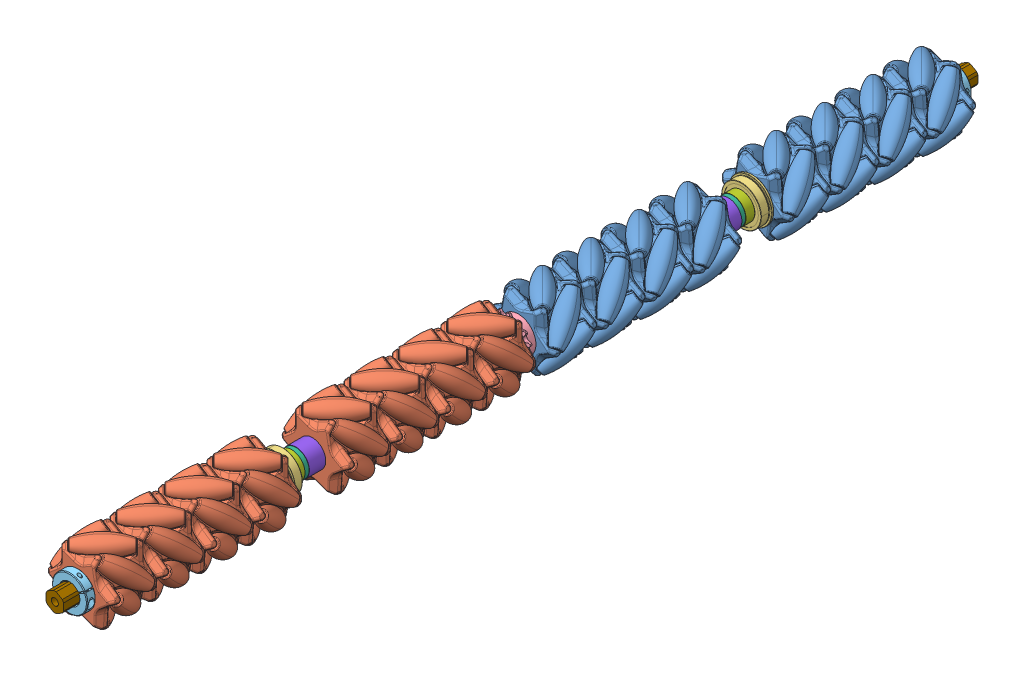
SolidWorks assembly rollers^IntakeBar, configuration Default. Lengths in mm.
Overall size (60.19 53.03 660.4).
28 component instances, 9 part files, 74 mates.
Components (placement in the parent):
- WCP-0125  Rev1-1: WCP-0125  Rev1 [Default] at (-38.2516 -1.4209 -91.9163) x (0 0 1) z (-1 0 0) size (40.13 53 60.19)
- WCP-0125  Rev1-2: WCP-0125  Rev1 [Default] at (-38.2516 -1.4209 -56.9913) x (0 0 1) z (-1 0 0) size (40.13 53 60.19)
- WCP-0125  Rev1-3: WCP-0125  Rev1 [Default] at (-38.2516 -1.4209 -22.0663) x (0 0 1) z (-1 0 0) size (40.13 53 60.19)
- WCP-0125  Rev1-4: WCP-0125  Rev1 [Default] at (-38.2516 -1.4209 -126.8412) x (0 0 1) z (-1 0 0) size (40.13 53 60.19)
- WCP-0125  Rev1-5: WCP-0125  Rev1 [Default] at (-38.2516 -1.4209 -225.933) x (0 0 1) z (-1 0 0) size (40.13 53 60.19)
- WCP-0125  Rev1-6: WCP-0125  Rev1 [Default] at (-38.2516 -1.4209 -295.783) x (0 0 1) z (-1 0 0) size (40.13 53 60.19)
- WCP-0125  Rev1-7: WCP-0125  Rev1 [Default] at (-38.2516 -1.4209 -191.008) x (0 0 1) z (-1 0 0) size (40.13 53 60.19)
- WCP-0125  Rev1-8: WCP-0125  Rev1 [Default] at (-38.2516 -1.4209 -260.858) x (0 0 1) z (-1 0 0) size (40.13 53 60.19)
- WCP-0126  Rev1-1: WCP-0126  Rev1 [Default] at (-38.2516 -1.4493 22.0345) x (0 0 -1) z (-1 0 0) size (40.13 53 60.19)
- WCP-0126  Rev1-2: WCP-0126  Rev1 [Default] at (-38.2516 -1.4493 56.9595) x (0 0 -1) z (-1 0 0) size (40.13 53 60.19)
- WCP-0126  Rev1-3: WCP-0126  Rev1 [Default] at (-38.2516 -1.4493 91.8845) x (0 0 -1) z (-1 0 0) size (40.13 53 60.19)
- WCP-0126  Rev1-4: WCP-0126  Rev1 [Default] at (-38.2516 -1.4493 126.8095) x (0 0 -1) z (-1 0 0) size (40.13 53 60.19)
- WCP-0126  Rev1-5: WCP-0126  Rev1 [Default] at (-38.2516 -1.4493 191.008) x (0 0 -1) z (-1 0 0) size (40.13 53 60.19)
- WCP-0126  Rev1-6: WCP-0126  Rev1 [Default] at (-38.2516 -1.4493 295.783) x (0 0 -1) z (-1 0 0) size (40.13 53 60.19)
- WCP-0126  Rev1-7: WCP-0126  Rev1 [Default] at (-38.2516 -1.4493 260.858) x (0 0 -1) z (-1 0 0) size (40.13 53 60.19)
- WCP-0126  Rev1-8: WCP-0126  Rev1 [Default] at (-38.2516 -1.4493 225.933) x (0 0 -1) z (-1 0 0) size (40.13 53 60.19)
- 13.75mm (1_2_ ThunderHex ID) x 1.125_ OD x 0.313_ WD (Flanged Bearing) (217-4006)-1: 13.75mm (1_2_ ThunderHex ID) x 1.125_ OD x 0.313_ WD (Flanged Bearing) (217-4006) [Default] at (-38.227 -1.4351 169.5768) x (-0.393668 0.919253 0) z (0 0 1) size (31.12 31.12 7.94)
- 16T Aluminum Hub Sprocket (#25 Chain, 1_2_ Hex Bore) (217-2642)-1: 16T Aluminum Hub Sprocket (#25 Chain, 1_2_ Hex Bore) (217-2642) [Default] at (-38.227 -1.4204 1.778) x (0.5 -0.866025 0) z (0 0 1) size (35.22 35.22 9.18)
- 13.75mm (1_2_ ThunderHex ID) x 1.125_ OD x 0.313_ WD (Flanged Bearing) (217-4006)-2: 13.75mm (1_2_ ThunderHex ID) x 1.125_ OD x 0.313_ WD (Flanged Bearing) (217-4006) [Default] at (-38.227 -1.4351 -169.5768) x (1 0 0) z (0 0 -1) size (31.12 31.12 7.94)
- WCP-0071 Clamping Split Shaft Collar.step-1: WCP-0071 Clamping Split Shaft Collar.step [Default] at (-38.227 -1.5524 316.4205) x (0.866025 0.5 0) z (0 0 1) size (25.38 25.4 6.35)
- WCP-0071 Clamping Split Shaft Collar.step-2: WCP-0071 Clamping Split Shaft Collar.step [Default] at (-38.3286 -1.4938 -316.4205) x (0.866025 -0.5 0) z (0 0 1) size (25.38 25.4 6.35)
- 1_8_ Acetal Spacer - 1_2_ Hex (217-2758)-1: 1_8_ Acetal Spacer - 1_2_ Hex (217-2758) [Default] at (-38.227 -1.3178 -157.6705) size (19.05 19.05 3.17)
- 1_4_ Acetal Spacer - 1_2_ Hex (217-3259)-1: 1_4_ Acetal Spacer - 1_2_ Hex (217-3259) [Default] at (-38.227 -1.3178 -162.433) x (0.866025 -0.5 0) z (0 0 1) size (19.5 19.5 6.35)
- 1_2_ Acetal Spacer - 1_2_ Hex (217-3261)-1: 1_2_ Acetal Spacer - 1_2_ Hex (217-3261) [Default] at (-38.0238 -1.4351 -149.733) x (0.866025 -0.5 0) z (0 0 1) size (19.5 19.5 12.7)
- 1_2_ Acetal Spacer - 1_2_ Hex (217-3261)-2: 1_2_ Acetal Spacer - 1_2_ Hex (217-3261) [Default] at (-38.227 -1.3178 149.733) x (0.866025 0.5 0) z (0 0 -1) size (19.5 19.5 12.7)
- 1_4_ Acetal Spacer - 1_2_ Hex (217-3259)-2: 1_4_ Acetal Spacer - 1_2_ Hex (217-3259) [Default] at (-38.227 -1.3178 162.433) x (0.866025 0.5 0) z (0 0 -1) size (19.5 19.5 6.35)
- 1_8_ Acetal Spacer - 1_2_ Hex (217-2758)-2: 1_8_ Acetal Spacer - 1_2_ Hex (217-2758) [Default] at (-38.227 -1.3178 157.6705) x (1 0 0) z (0 0 -1) size (19.05 19.05 3.17)
- ThunderHexShaft-1: ThunderHexShaft [Default] at (-38.227 -1.4351 0) x (0.866025 -0.5 0) z (0 0 1) size (13.74 12.75 660.4)
Mates (geometry in assembly coordinates):
- Coincident12: coincident anti-aligned: plane of WCP-0125  Rev1-1 through (-38.2516 -1.4209 -109.3787) normal (0 0 -1); plane of WCP-0125  Rev1-4 through (-38.2516 -1.4209 -109.3787) normal (0 0 1)
- Coincident13: coincident anti-aligned: plane of WCP-0125  Rev1-1 through (-38.2516 -1.4209 -74.4537) normal (0 0 1); plane of WCP-0125  Rev1-2 through (-38.2516 -1.4209 -74.4537) normal (0 0 -1)
- Coincident14: coincident anti-aligned: plane of WCP-0125  Rev1-2 through (-38.2516 -1.4209 -39.5288) normal (0 0 1); plane of WCP-0125  Rev1-3 through (-38.2516 -1.4209 -39.5288) normal (0 0 -1)
- Coincident103: coincident anti-aligned: plane of WCP-0125  Rev1-3 through (-38.2516 -1.4209 -4.6037) normal (0 0 1); plane of 16T Aluminum Hub Sprocket (#25 Chain, 1_2_ Hex Bore) (217-2642)-1 through (-38.227 -1.4204 -4.6037) normal (0 0 -1)
- Coincident70: coincident anti-aligned: plane of WCP-0125  Rev1-5 through (-38.2516 -1.4209 -243.3955) normal (0 0 -1); plane of WCP-0125  Rev1-8 through (-38.2516 -1.4209 -243.3955) normal (0 0 1)
- Coincident71: coincident anti-aligned: plane of WCP-0125  Rev1-5 through (-38.2516 -1.4209 -208.4705) normal (0 0 1); plane of WCP-0125  Rev1-7 through (-38.2516 -1.4209 -208.4705) normal (0 0 -1)
- Coincident69: coincident anti-aligned: plane of WCP-0125  Rev1-6 through (-38.2516 -1.4209 -278.3205) normal (0 0 1); plane of WCP-0125  Rev1-8 through (-38.2516 -1.4209 -278.3205) normal (0 0 -1)
- Coincident147: coincident anti-aligned: plane of WCP-0125  Rev1-6 through (-38.2516 -1.4209 -313.2455) normal (0 0 -1); plane of WCP-0071 Clamping Split Shaft Collar.step-2 through (-38.3286 -1.4938 -313.2455) normal (0 0 1)
- Coincident105: coincident anti-aligned: plane of WCP-0125  Rev1-7 through (-38.2516 -1.4209 -173.5455) normal (0 0 1); plane of 13.75mm (1_2_ ThunderHex ID) x 1.125_ OD x 0.313_ WD (Flanged Bearing) (217-4006)-2 through (-38.227 -16.9951 -173.5455) normal (0 0 -1)
- Coincident20: coincident anti-aligned: plane of WCP-0126  Rev1-1 through (-38.2516 -1.4493 39.497) normal (0 0 1); plane of WCP-0126  Rev1-2 through (-38.2516 -1.4493 39.497) normal (0 0 -1)
- Coincident102: coincident anti-aligned: plane of WCP-0126  Rev1-1 through (-38.2516 -1.4493 4.572) normal (0 0 -1); plane of 16T Aluminum Hub Sprocket (#25 Chain, 1_2_ Hex Bore) (217-2642)-1 through (-38.227 -1.4204 4.572) normal (0 0 1)
- Coincident26: coincident anti-aligned: plane of WCP-0126  Rev1-2 through (-38.2516 -1.4493 74.422) normal (0 0 1); plane of WCP-0126  Rev1-3 through (-38.2516 -1.4493 74.422) normal (0 0 -1)
- Coincident21: coincident anti-aligned: plane of WCP-0126  Rev1-3 through (-38.2516 -1.4493 109.347) normal (0 0 1); plane of WCP-0126  Rev1-4 through (-38.2516 -1.4493 109.347) normal (0 0 -1)
- Coincident91: coincident anti-aligned: plane of WCP-0126  Rev1-5 through (-38.2516 -1.4493 208.4705) normal (0 0 1); plane of WCP-0126  Rev1-8 through (-38.2516 -1.4493 208.4705) normal (0 0 -1)
- Coincident106: coincident anti-aligned: plane of WCP-0126  Rev1-5 through (-38.2516 -1.4493 173.5455) normal (0 0 -1); plane of 13.75mm (1_2_ ThunderHex ID) x 1.125_ OD x 0.313_ WD (Flanged Bearing) (217-4006)-1 through (-52.5306 -7.5606 173.5455) normal (0 0 1)
- Coincident92: coincident anti-aligned: plane of WCP-0126  Rev1-6 through (-38.2516 -1.4493 278.3205) normal (0 0 -1); plane of WCP-0126  Rev1-7 through (-38.2516 -1.4493 278.3205) normal (0 0 1)
- Coincident150: coincident anti-aligned: plane of WCP-0126  Rev1-6 through (-38.2516 -1.4493 313.2455) normal (0 0 1); plane of WCP-0071 Clamping Split Shaft Collar.step-1 through (-38.227 -1.5524 313.2455) normal (0 0 -1)
- Coincident93: coincident anti-aligned: plane of WCP-0126  Rev1-7 through (-38.2516 -1.4493 243.3955) normal (0 0 -1); plane of WCP-0126  Rev1-8 through (-38.2516 -1.4493 243.3955) normal (0 0 1)
- Coincident229: coincident anti-aligned: plane of 13.75mm (1_2_ ThunderHex ID) x 1.125_ OD x 0.313_ WD (Flanged Bearing) (217-4006)-1 through (-44.5469 -4.1416 165.608) normal (0 0 -1); plane of 1_4_ Acetal Spacer - 1_2_ Hex (217-3259)-2 through (-38.227 -1.3178 165.608) normal (0 0 1)
- Coincident216: coincident anti-aligned: plane of 13.75mm (1_2_ ThunderHex ID) x 1.125_ OD x 0.313_ WD (Flanged Bearing) (217-4006)-2 through (-38.227 -8.3101 -165.608) normal (0 0 1); plane of 1_4_ Acetal Spacer - 1_2_ Hex (217-3259)-1 through (-38.227 -1.3178 -165.608) normal (0 0 -1)
- Coincident212: coincident anti-aligned: plane of 1_8_ Acetal Spacer - 1_2_ Hex (217-2758)-1 through (-38.227 -1.3178 -156.083) normal (0 0 1); plane of 1_2_ Acetal Spacer - 1_2_ Hex (217-3261)-1 through (-38.0238 -1.4351 -156.083) normal (0 0 -1)
- Coincident213: coincident anti-aligned: plane of 1_8_ Acetal Spacer - 1_2_ Hex (217-2758)-1 through (-38.227 -1.3178 -159.258) normal (0 0 -1); plane of 1_4_ Acetal Spacer - 1_2_ Hex (217-3259)-1 through (-38.227 -1.3178 -159.258) normal (0 0 1)
- Coincident224: coincident anti-aligned: plane of 1_2_ Acetal Spacer - 1_2_ Hex (217-3261)-2 through (-38.227 -1.3178 156.083) normal (0 0 1); plane of 1_8_ Acetal Spacer - 1_2_ Hex (217-2758)-2 through (-38.227 -1.3178 156.083) normal (0 0 -1)
- Coincident225: coincident anti-aligned: plane of 1_4_ Acetal Spacer - 1_2_ Hex (217-3259)-2 through (-38.227 -1.3178 159.258) normal (0 0 -1); plane of 1_8_ Acetal Spacer - 1_2_ Hex (217-2758)-2 through (-38.227 -1.3178 159.258) normal (0 0 1)
- Coincident252: coincident anti-aligned: plane of ThunderHexShaft-1 through (-31.8516 -5.1159 457.2) normal (1 0 0); plane of WCP-0125  Rev1-1 through (-31.8516 -5.1159 -15.7163) normal (-1 0 0)
- Coincident253: coincident anti-aligned: plane of ThunderHexShaft-1 through (-38.227 -8.7968 457.2) normal (0.5 -0.866025 0); plane of WCP-0125  Rev1-1 through (-38.2516 -8.811 -15.7163) normal (-0.5 0.866025 0)
- Coincident254: coincident anti-aligned: plane of ThunderHexShaft-1 through (-31.8516 -5.1159 457.2) normal (1 0 0); plane of WCP-0125  Rev1-2 through (-31.8516 -5.1159 19.2087) normal (-1 0 0)
- Coincident255: coincident anti-aligned: plane of ThunderHexShaft-1 through (-38.227 -8.7968 457.2) normal (0.5 -0.866025 0); plane of WCP-0125  Rev1-2 through (-38.2516 -8.811 19.2087) normal (-0.5 0.866025 0)
- Coincident256: coincident anti-aligned: plane of ThunderHexShaft-1 through (-31.8516 -5.1159 457.2) normal (1 0 0); plane of WCP-0125  Rev1-3 through (-31.8516 -5.1159 54.1337) normal (-1 0 0)
- Coincident257: coincident anti-aligned: plane of ThunderHexShaft-1 through (-38.227 -8.7968 457.2) normal (0.5 -0.866025 0); plane of WCP-0125  Rev1-3 through (-38.2516 -8.811 54.1337) normal (-0.5 0.866025 0)
- Coincident258: coincident anti-aligned: plane of ThunderHexShaft-1 through (-31.8516 -5.1159 457.2) normal (1 0 0); plane of WCP-0125  Rev1-4 through (-31.8516 -5.1159 -50.6412) normal (-1 0 0)
- Coincident259: coincident anti-aligned: plane of ThunderHexShaft-1 through (-38.227 -8.7968 457.2) normal (0.5 -0.866025 0); plane of WCP-0125  Rev1-4 through (-38.2516 -8.811 -50.6412) normal (-0.5 0.866025 0)
- Coincident260: coincident anti-aligned: plane of ThunderHexShaft-1 through (-31.8516 -5.1159 457.2) normal (1 0 0); plane of WCP-0125  Rev1-5 through (-31.8516 -5.1159 -149.733) normal (-1 0 0)
- Coincident261: coincident anti-aligned: plane of ThunderHexShaft-1 through (-38.227 -8.7968 457.2) normal (0.5 -0.866025 0); plane of WCP-0125  Rev1-5 through (-38.2516 -8.811 -149.733) normal (-0.5 0.866025 0)
- Coincident262: coincident anti-aligned: plane of ThunderHexShaft-1 through (-31.8516 -5.1159 457.2) normal (1 0 0); plane of WCP-0125  Rev1-6 through (-31.8516 -5.1159 -219.583) normal (-1 0 0)
- Coincident263: coincident anti-aligned: plane of ThunderHexShaft-1 through (-38.227 -8.7968 457.2) normal (0.5 -0.866025 0); plane of WCP-0125  Rev1-6 through (-38.2516 -8.811 -219.583) normal (-0.5 0.866025 0)
- Coincident264: coincident anti-aligned: plane of ThunderHexShaft-1 through (-31.8516 -5.1159 457.2) normal (1 0 0); plane of WCP-0125  Rev1-7 through (-31.8516 -5.1159 -114.808) normal (-1 0 0)
- Coincident265: coincident anti-aligned: plane of ThunderHexShaft-1 through (-38.227 -8.7968 457.2) normal (0.5 -0.866025 0); plane of WCP-0125  Rev1-7 through (-38.2516 -8.811 -114.808) normal (-0.5 0.866025 0)
- Coincident266: coincident anti-aligned: plane of ThunderHexShaft-1 through (-31.8516 -5.1159 457.2) normal (1 0 0); plane of WCP-0125  Rev1-8 through (-31.8516 -5.1159 -184.658) normal (-1 0 0)
- Coincident267: coincident anti-aligned: plane of ThunderHexShaft-1 through (-38.227 -8.7968 457.2) normal (0.5 -0.866025 0); plane of WCP-0125  Rev1-8 through (-38.2516 -8.811 -184.658) normal (-0.5 0.866025 0)
- Coincident268: coincident anti-aligned: plane of ThunderHexShaft-1 through (-31.8516 -5.1159 457.2) normal (1 0 0); plane of WCP-0126  Rev1-1 through (-31.8516 2.2457 98.2345) normal (-1 0 0)
- Coincident269: coincident anti-aligned: plane of ThunderHexShaft-1 through (-31.8516 2.2457 457.2) normal (0.5 0.866025 0); plane of WCP-0126  Rev1-1 through (-38.2516 5.9408 98.2345) normal (-0.5 -0.866025 0)
- Coincident270: coincident anti-aligned: plane of ThunderHexShaft-1 through (-31.8516 -5.1159 457.2) normal (1 0 0); plane of WCP-0126  Rev1-2 through (-31.8516 2.2457 133.1595) normal (-1 0 0)
- Coincident271: coincident anti-aligned: plane of ThunderHexShaft-1 through (-31.8516 2.2457 457.2) normal (0.5 0.866025 0); plane of WCP-0126  Rev1-2 through (-38.2516 5.9408 133.1595) normal (-0.5 -0.866025 0)
- Coincident272: coincident anti-aligned: plane of ThunderHexShaft-1 through (-31.8516 -5.1159 457.2) normal (1 0 0); plane of WCP-0126  Rev1-3 through (-31.8516 2.2457 168.0845) normal (-1 0 0)
- Coincident273: coincident anti-aligned: plane of ThunderHexShaft-1 through (-31.8516 2.2457 457.2) normal (0.5 0.866025 0); plane of WCP-0126  Rev1-3 through (-38.2516 5.9408 168.0845) normal (-0.5 -0.866025 0)
- Coincident274: coincident anti-aligned: plane of ThunderHexShaft-1 through (-31.8516 -5.1159 457.2) normal (1 0 0); plane of WCP-0126  Rev1-4 through (-31.8516 2.2457 203.0095) normal (-1 0 0)
- Coincident275: coincident anti-aligned: plane of ThunderHexShaft-1 through (-31.8516 2.2457 457.2) normal (0.5 0.866025 0); plane of WCP-0126  Rev1-4 through (-38.2516 5.9408 203.0095) normal (-0.5 -0.866025 0)
- Coincident277: coincident anti-aligned: plane of ThunderHexShaft-1 through (-31.8516 -5.1159 457.2) normal (1 0 0); plane of WCP-0126  Rev1-5 through (-31.8516 2.2457 267.208) normal (-1 0 0)
- Coincident278: coincident anti-aligned: plane of ThunderHexShaft-1 through (-31.8516 2.2457 457.2) normal (0.5 0.866025 0); plane of WCP-0126  Rev1-5 through (-38.2516 5.9408 267.208) normal (-0.5 -0.866025 0)
- Coincident279: coincident anti-aligned: plane of ThunderHexShaft-1 through (-31.8516 -5.1159 457.2) normal (1 0 0); plane of WCP-0126  Rev1-6 through (-31.8516 2.2457 371.983) normal (-1 0 0)
- Coincident280: coincident anti-aligned: plane of ThunderHexShaft-1 through (-31.8516 2.2457 457.2) normal (0.5 0.866025 0); plane of WCP-0126  Rev1-6 through (-38.2516 5.9408 371.983) normal (-0.5 -0.866025 0)
- Coincident281: coincident anti-aligned: plane of ThunderHexShaft-1 through (-31.8516 -5.1159 457.2) normal (1 0 0); plane of WCP-0126  Rev1-7 through (-31.8516 2.2457 337.058) normal (-1 0 0)
- Coincident282: coincident anti-aligned: plane of ThunderHexShaft-1 through (-31.8516 2.2457 457.2) normal (0.5 0.866025 0); plane of WCP-0126  Rev1-7 through (-38.2516 5.9408 337.058) normal (-0.5 -0.866025 0)
- Coincident283: coincident anti-aligned: plane of ThunderHexShaft-1 through (-31.8516 -5.1159 457.2) normal (1 0 0); plane of WCP-0126  Rev1-8 through (-31.8516 2.2457 302.133) normal (-1 0 0)
- Coincident284: coincident anti-aligned: plane of ThunderHexShaft-1 through (-31.8516 2.2457 457.2) normal (0.5 0.866025 0); plane of WCP-0126  Rev1-8 through (-38.2516 5.9408 302.133) normal (-0.5 -0.866025 0)
- Coincident287: coincident anti-aligned: plane of ThunderHexShaft-1 through (-38.227 5.9266 457.2) normal (-0.5 0.866025 0); plane of 16T Aluminum Hub Sprocket (#25 Chain, 1_2_ Hex Bore) (217-2642)-1 through (-38.227 5.9266 -4.6048) normal (0.5 -0.866025 0)
- Coincident288: coincident anti-aligned: plane of ThunderHexShaft-1 through (-31.8516 2.2457 457.2) normal (0.5 0.866025 0); plane of 16T Aluminum Hub Sprocket (#25 Chain, 1_2_ Hex Bore) (217-2642)-1 through (-31.8643 2.2531 -4.6048) normal (-0.5 -0.866025 0)
- Coincident291: coincident anti-aligned: plane of ThunderHexShaft-1 through (-38.227 5.9266 457.2) normal (-0.5 0.866025 0); plane of WCP-0071 Clamping Split Shaft Collar.step-1 through (-38.227 5.9266 313.2455) normal (0.5 -0.866025 0)
- Coincident292: coincident anti-aligned: plane of ThunderHexShaft-1 through (-31.8516 2.2457 457.2) normal (0.5 0.866025 0); plane of WCP-0071 Clamping Split Shaft Collar.step-1 through (-31.75 2.1871 313.2455) normal (-0.5 -0.866025 0)
- Coincident293: coincident anti-aligned: plane of ThunderHexShaft-1 through (-31.8516 2.2457 457.2) normal (0.5 0.866025 0); plane of WCP-0071 Clamping Split Shaft Collar.step-2 through (-31.8516 2.2457 -319.5955) normal (-0.5 -0.866025 0)
- Coincident294: coincident anti-aligned: plane of ThunderHexShaft-1 through (-31.8516 -5.1159 457.2) normal (1 0 0); plane of WCP-0071 Clamping Split Shaft Collar.step-2 through (-31.8516 -5.2333 -319.5955) normal (-1 0 0)
- Coincident295: coincident anti-aligned: plane of ThunderHexShaft-1 through (-44.6024 -5.1159 457.2) normal (-0.5 -0.866025 0); plane of 1_8_ Acetal Spacer - 1_2_ Hex (217-2758)-1 through (-44.704 -5.0573 -156.083) normal (0.5 0.866025 0)
- Coincident296: coincident anti-aligned: plane of ThunderHexShaft-1 through (-38.227 -8.7968 457.2) normal (0.5 -0.866025 0); plane of 1_8_ Acetal Spacer - 1_2_ Hex (217-2758)-1 through (-38.227 -8.7968 -156.083) normal (-0.5 0.866025 0)
- Coincident297: coincident anti-aligned: plane of ThunderHexShaft-1 through (-44.6024 -5.1159 457.2) normal (-0.5 -0.866025 0); plane of 1_4_ Acetal Spacer - 1_2_ Hex (217-3259)-1 through (-44.704 -5.0573 -159.258) normal (0.5 0.866025 0)
- Coincident298: coincident anti-aligned: plane of ThunderHexShaft-1 through (-38.227 -8.7968 457.2) normal (0.5 -0.866025 0); plane of 1_4_ Acetal Spacer - 1_2_ Hex (217-3259)-1 through (-38.227 -8.7968 -159.258) normal (-0.5 0.866025 0)
- Coincident299: coincident anti-aligned: plane of ThunderHexShaft-1 through (-44.6024 -5.1159 457.2) normal (-0.5 -0.866025 0); plane of 1_2_ Acetal Spacer - 1_2_ Hex (217-3261)-1 through (-44.5008 -5.1746 -143.383) normal (0.5 0.866025 0)
- Coincident300: coincident anti-aligned: plane of ThunderHexShaft-1 through (-38.227 5.9266 457.2) normal (-0.5 0.866025 0); plane of 1_2_ Acetal Spacer - 1_2_ Hex (217-3261)-1 through (-38.0238 6.0439 -143.383) normal (0.5 -0.866025 0)
- Coincident301: coincident anti-aligned: plane of ThunderHexShaft-1 through (-38.227 -8.7968 457.2) normal (0.5 -0.866025 0); plane of 1_2_ Acetal Spacer - 1_2_ Hex (217-3261)-2 through (-31.75 -5.0573 143.383) normal (-0.5 0.866025 0)
- Coincident302: coincident anti-aligned: plane of ThunderHexShaft-1 through (-44.6024 -5.1159 457.2) normal (-0.5 -0.866025 0); plane of 1_2_ Acetal Spacer - 1_2_ Hex (217-3261)-2 through (-38.227 -8.7968 143.383) normal (0.5 0.866025 0)
- Coincident303: coincident anti-aligned: plane of ThunderHexShaft-1 through (-44.6024 -5.1159 457.2) normal (-0.5 -0.866025 0); plane of 1_4_ Acetal Spacer - 1_2_ Hex (217-3259)-2 through (-38.227 -8.7968 159.258) normal (0.5 0.866025 0)
- Coincident304: coincident anti-aligned: plane of ThunderHexShaft-1 through (-38.227 -8.7968 457.2) normal (0.5 -0.866025 0); plane of 1_4_ Acetal Spacer - 1_2_ Hex (217-3259)-2 through (-31.75 -5.0573 159.258) normal (-0.5 0.866025 0)
- Coincident305: coincident anti-aligned: plane of ThunderHexShaft-1 through (-44.6024 -5.1159 457.2) normal (-0.5 -0.866025 0); plane of 1_8_ Acetal Spacer - 1_2_ Hex (217-2758)-2 through (-38.227 -8.7968 156.083) normal (0.5 0.866025 0)
- Coincident306: coincident anti-aligned: plane of ThunderHexShaft-1 through (-38.227 -8.7968 457.2) normal (0.5 -0.866025 0); plane of 1_8_ Acetal Spacer - 1_2_ Hex (217-2758)-2 through (-31.75 -5.0573 156.083) normal (-0.5 0.866025 0)
